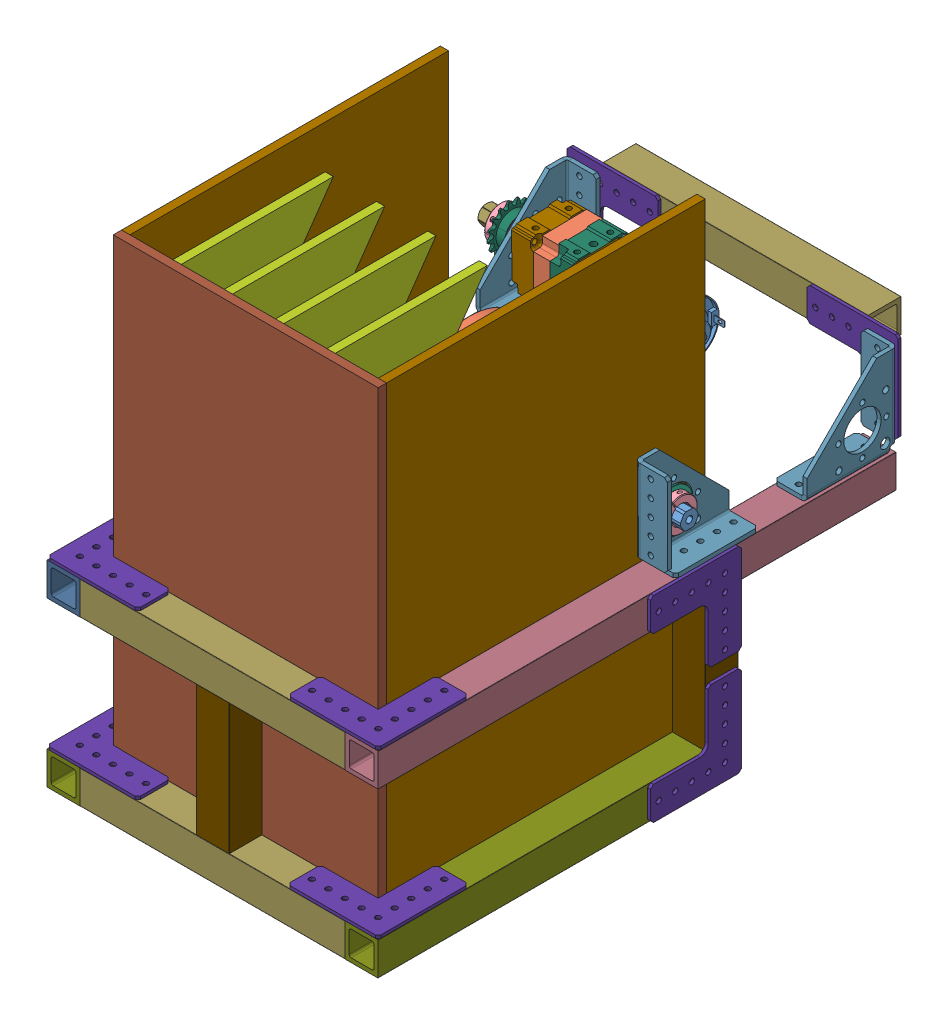
SolidWorks assembly Outtake, configuration Default. Lengths in mm.
Overall size (762 627.63 736.73).
92 component instances, 37 part files, 6 mates.
Components (placement in the parent):
- Skeleton Infinite Recharge Sketch-1: Skeleton Infinite Recharge Sketch [Default] at origin size (762 246.63 736.6)
- Assem_Launch_Component(wheels,hexshaft,motor,etc.)-SP - Copy-1: Assem_Launch_Component(wheels,hexshaft,motor,etc.)-SP - Copy [Default] at (101.6 246.634 342.9) size (290.76 381 426.56)
  - ThunderHex(.5 11inch)-SP-1: ThunderHex(.5 11inch)-SP [Default] at (-34.4752 190.5 -222.25) x (0 0.015634 -0.999878) z (-1 0 0) size (13.74 12.75 279.4)
  - CompliantWheel(4inch 500)SP-1: CompliantWheel(4inch 500)SP [Default] at (-57.548 185.9668 -238.3103) x (0 -0.486399 -0.873737) z (-1 0 0) size (101.6 101.6 25.4)
    - CompliantWheel(4inch 500)SP.STEP-1: CompliantWheel(4inch 500)SP.STEP [Default] at origin size (101.6 101.6 25.4)
      - 4IN Compliant Wheel FINAL Overmold.STEP-1: 4IN Compliant Wheel FINAL Overmold.STEP [Default] at (-16.2374 3.8509 18.652) size (101.6 101.6 25.4)
      - 2in Wheel Intergrated 0500 HEX Hub.STEP-1: 2in Wheel Intergrated 0500 HEX Hub.STEP [Default] at (-16.2374 3.8509 5.952) x (-1 0 0) z (0 0 -1) size (41.91 41.91 25.4)
  - CompliantWheel(4inch 500)SP.STEP-1: CompliantWheel(4inch 500)SP.STEP [Default] at (-82.948 195.0332 -206.1897) x (0 0.486399 0.873737) z (-1 0 0) size (101.6 101.6 25.4)
    - 4IN Compliant Wheel FINAL Overmold.STEP-1: 4IN Compliant Wheel FINAL Overmold.STEP [Default] at (-16.2374 3.8509 18.652) size (101.6 101.6 25.4)
    - 2in Wheel Intergrated 0500 HEX Hub.STEP-1: 2in Wheel Intergrated 0500 HEX Hub.STEP [Default] at (-16.2374 3.8509 5.952) x (-1 0 0) z (0 0 -1) size (41.91 41.91 25.4)
  - CompliantWheel(4inch 500)SP.STEP-3: CompliantWheel(4inch 500)SP.STEP [Default] at (-108.348 195.2838 -206.2625) x (0 0.5 0.866025) z (-1 0 0) size (101.6 101.6 25.4)
    - 4IN Compliant Wheel FINAL Overmold.STEP-1: 4IN Compliant Wheel FINAL Overmold.STEP [Default] at (-16.2374 3.8509 18.652) size (101.6 101.6 25.4)
    - 2in Wheel Intergrated 0500 HEX Hub.STEP-1: 2in Wheel Intergrated 0500 HEX Hub.STEP [Default] at (-16.2374 3.8509 5.952) x (-1 0 0) z (0 0 -1) size (41.91 41.91 25.4)
  - CompliantWheel(4inch 500)SP.STEP-4: CompliantWheel(4inch 500)SP.STEP [Default] at (-133.748 195.0332 -206.1897) x (0 0.486399 0.873737) z (-1 0 0) size (101.6 101.6 25.4)
    - 4IN Compliant Wheel FINAL Overmold.STEP-1: 4IN Compliant Wheel FINAL Overmold.STEP [Default] at (-16.2374 3.8509 18.652) size (101.6 101.6 25.4)
    - 2in Wheel Intergrated 0500 HEX Hub.STEP-1: 2in Wheel Intergrated 0500 HEX Hub.STEP [Default] at (-16.2374 3.8509 5.952) x (-1 0 0) z (0 0 -1) size (41.91 41.91 25.4)
  - ClampingShaftCollar(.5 in)SP-1: ClampingShaftCollar(.5 in)SP [Default] at (-47.625 190.7032 -222.2468) x (0 0.015634 -0.999878) z (-1 0 0) size (25.39 25.4 6.35)
  - ClampingShaftCollar(.5 in)SP-2: ClampingShaftCollar(.5 in)SP [Default] at (-155.575 190.4012 -222.4275) x (0 0.873737 -0.486399) z (-1 0 0) size (25.39 25.4 6.35)
  - VersaPlanetaryv2_Single_Stage_10_1_with_775_Series (General_GearBox_Shell)-SP-1: VersaPlanetaryv2_Single_Stage_10_1_with_775_Series (General_GearBox_Shell)-SP [Default] at (-205.875 214.6824 -345.637) x (-1 0 0) z (0 -0.015634 0.999878) size (166.6 51.28 52.65)
    - VersaPlanetary_v2_Single_Stage_10_1_with_775_Series (General_GearBox_Shell)-SP.STEP-1: VersaPlanetary_v2_Single_Stage_10_1_with_775_Series (General_GearBox_Shell)-SP.STEP [Default] at origin size (166.6 51.28 52.65)
      - 217-2820 Rev1_Public.STEP-1: 217-2820 Rev1_Public.STEP [Default] at (-4.6546 22.225 0) x (0 -0.456494 0.889726) z (-1 0 0) size (39.22 38.88 17.4)
        - 217-2625-100.STEP-1: 217-2625-100.STEP [Default] at origin size (39.22 38.88 12.7)
          - 217-2625-008 Rev1.STEP-1: 217-2625-008 Rev1.STEP [Default] at origin size (34.7 34.7 4.7)
          - 217-2625-010 Rev1.STEP-1: 217-2625-010 Rev1.STEP [Default] at (0 10.193 3.65) x (0.999813 0.019336 0) z (0 0 1) size (4 4 12)
          - 217-2625-010 Rev1.STEP-2: 217-2625-010 Rev1.STEP [Default] at (8.691 -5.3258 3.65) size (4 4 12)
          - 217-2625-010 Rev1.STEP-3: 217-2625-010 Rev1.STEP [Default] at (-8.691 -5.3258 3.65) size (4 4 12)
          - 217-2625-005 Rev1_Planet_Revolving_Follower01.STEP-1: 217-2625-005 Rev1_Planet_Revolving_Follower01.STEP [Default] at (8.691 -5.3258 6.35) x (0.932816 0.360354 0) z (0 0 1) size (16.89 16.89 8)
          - 217-2625-005 Rev1_Planet_Revolving_Follower01.STEP-2: 217-2625-005 Rev1_Planet_Revolving_Follower01.STEP [Default] at (-8.691 -5.3258 6.35) x (-0.932788 -0.360426 0) z (0 0 1) size (16.89 16.89 8)
          - 217-2625-005 Rev1_Planet_Revolving_Follower01.STEP-3: 217-2625-005 Rev1_Planet_Revolving_Follower01.STEP [Default] at (0 10.193 6.35) x (0.893583 0.448898 0) z (0 0 1) size (16.89 16.89 8)
        - 217-2625-007 Rev1_Public.STEP-1: 217-2625-007 Rev1_Public.STEP [Default] at (0 0 6.7) x (0.992772 0.120019 0) z (0 0 1) size (15.27 15.27 12.7)
      - 217-2625-026 Rev1.STEP-1: 217-2625-026 Rev1.STEP [Default] at (-6.5 22.225 0) x (0 -1 0) z (-1 0 0) size (44.45 42 18.12)
      - 217-2742-001 Rev4.STEP-1: 217-2742-001 Rev4.STEP [Default] at (0.2002 22.225 0) x (1 0 0) z (0 -0.092627 0.995701) size (7 28 28)
      - 217-2742-001 Rev4.STEP-2: 217-2742-001 Rev4.STEP [Default] at (8.2002 22.225 0) size (7 28 28)
      - 217-2625-017 Rev1_9714K61.STEP-1: 217-2625-017 Rev1_9714K61.STEP [Default] at (7.42 22.3002 -0.342) x (0 0.56703 0.823697) z (0 -0.823697 0.56703) size (28.51 4.98 27.43)
      - 217-2625-003 Rev1.STEP-1: 217-2625-003 Rev1.STEP [Default] at (7.4478 22.225 0) x (0 -1 0) z (1 0 0) size (17 17 64.11)
      - 217-2625-018 Rev1_98541A410.STEP-1: 217-2625-018 Rev1_98541A410.STEP [Default] at (-0.7046 22.225 0) x (1 0 0) z (0 -0.017452 0.999848) size (1 19.6 17.4)
      - 832-1750-Ring-Gear-Screw_SSA0832-0500ZC.STEP-1: 832-1750-Ring-Gear-Screw_SSA0832-0500ZC.STEP [Default] at (-30.7 4.725 -17.5) x (0 0.997447 0.071411) z (0 -0.071411 0.997447) size (6.73 48.51 6.73)
      - 832-1750-Ring-Gear-Screw_SSA0832-0500ZC.STEP-2: 832-1750-Ring-Gear-Screw_SSA0832-0500ZC.STEP [Default] at (-30.7 39.725 17.5) x (0 0.005929 0.999982) z (0 -0.999982 0.005929) size (6.73 48.51 6.73)
      - 217-2625-025 Rev1.STEP-1: 217-2625-025 Rev1.STEP [Default] at (-23.2 22.225 0) x (0 -1 0) z (-1 0 0) size (44.45 42 18)
      - 217-4649-002 Rev1_SSA0832-0500ZC.STEP-1: 217-4649-002 Rev1_SSA0832-0500ZC.STEP [Default] at (-34.2 4.2645 17.9605) x (0 0.33842 -0.940995) z (0 0.940995 0.33842) size (6.73 16.76 6.73)
      - 217-4649-002 Rev1_SSA0832-0500ZC.STEP-2: 217-4649-002 Rev1_SSA0832-0500ZC.STEP [Default] at (-34.2 40.1855 -17.9605) x (0 -0.308932 -0.951084) z (0 0.951084 -0.308932) size (6.73 16.76 6.73)
      - 217-4649-006 Rev1_SSA0004-008BA.STEP-1: 217-4649-006 Rev1_SSA0004-008BA.STEP [Default] at (-30.7 22.225 14.5) x (0 0.5 -0.866025) z (0 -0.866025 -0.5) size (7 14 7)
      - 217-4649-006 Rev1_SSA0004-008BA.STEP-2: 217-4649-006 Rev1_SSA0004-008BA.STEP [Default] at (-30.7 22.225 -14.5) x (0 -1 0) z (0 0 1) size (7 14 7)
      - 217-2822-002 Rev4.STEP-1: 217-2822-002 Rev4.STEP [Default] at (-32.45 22.225 0) x (0 -1 0) z (-1 0 0) size (42 42 5.3)
      - 217-4347-000 Rev1.STEP-1: 217-4347-000 Rev1.STEP [Default] at (-34.2 22.225 0) x (-1 0 0) z (0 1 0) size (88 44.3 44.3)
      - 217-2816-001 Rev1.STEP-1: 217-2816-001 Rev1.STEP [Default] at (-6.35 22.225 0) x (0 -1 0) z (1 0 0) size (42 42 14.51)
      - 217-4649-001 Rev1.STEP-1: 217-4649-001 Rev1.STEP [Default] at (-20.554 22.225 0) x (0 -1 0) z (1 0 0) size (18 18 13)
      - 217-4649-007 Rev1_94105A824.STEP-1: 217-4649-007 Rev1_94105A824.STEP [Default] at (-26.029 22.225 -6.7835) x (-0.996104 -0.088191 0) z (0 0 -1) size (4.83 4.83 4.77)
      - 217-2625-013 Rev2.STEP-1: 217-2625-013 Rev2.STEP [Default] at (-25.2898 22.225 0) x (0 0 1) z (-1 0 0) size (8.01 7.94 7.5)
  - 13_75mm_1_2_ThunderHex_ID_x_1_125_OD_x_0_313_WD_Flanged_Bearing_217-4006.step-1: 13_75mm_1_2_ThunderHex_ID_x_1_125_OD_x_0_313_WD_Flanged_Bearing_217-4006.step [Default] at (-0.3489 190.5 -222.25) x (0 -0.574166 -0.818739) z (1 0 0) size (31.12 31.12 7.94)
  - betterRamp RC-1: betterRamp RC [Default] at (-39.37 168.0882 -127) x (-1 0 0) z (0 0 -1) size (6.35 381 215.9)
  - betterRamp RC-2: betterRamp RC [Default] at (-118.11 168.0882 -127) x (-1 0 0) z (0 0 -1) size (6.35 381 215.9)
  - betterRamp RC-3: betterRamp RC [Default] at (-78.74 168.0882 -127) x (-1 0 0) z (0 0 -1) size (6.35 381 215.9)
  - betterRamp RC-4: betterRamp RC [Default] at (-157.48 168.0882 -127) x (-1 0 0) z (0 0 -1) size (6.35 381 215.9)
  - ClampingShaftCollar(.5 in)SP-3: ClampingShaftCollar(.5 in)SP [Default] at (6.9517 190.5 -222.25) x (0 0.858103 0.513478) z (-1 0 0) size (25.39 25.4 6.35)
  - ThunderHexFlangedBearing(0.5in) RC-1: ThunderHexFlangedBearing(0.5in) RC [Default] at (-203.9473 190.5 -222.25) x (0 0.030565 0.999533) z (-1 0 0) size (31.12 31.12 7.94)
  - ClampingShaftCollar(.5 in)SP-4: ClampingShaftCollar(.5 in)SP [Default] at (-209.7506 190.5 -222.25) x (0 -0.581767 0.813355) z (-1 0 0) size (25.39 25.4 6.35)
  - Wall(15 by 15 in .125thickness)-SP-2: Wall(15 by 15 in .125thickness)-SP [Default] at (0 190.5 -128.5875) x (-1 0 0) z (0 0 -1) size (6.35 381 244.47)
  - Wall(15 by 15 in .125thickness)-SP-3: Wall(15 by 15 in .125thickness)-SP [Default] at (-203.2 190.5 -128.5875) x (1 0 0) z (0 0 -1) size (6.35 381 244.47)
  - 1x1AluminumStock(15in)-1: 1x1AluminumStock(15in) [Default] at (-228.6 139.7 -1803.4) size (25.4 25.4 419.1)
  - BackWall-SP-1: BackWall-SP [Default] at (311.6896 672.1897 -6.35) size (203.2 381 6.35)
  - 1x1AluminumStock(9.5in)-1: 1x1AluminumStock(9.5in) [Default] at (1625.6 139.7 0) x (0 0 1) z (-1 0 0) size (25.4 25.4 203.2)
  - 1x1AluminumStock(9.5in)-2: 1x1AluminumStock(9.5in) [Default] at (1625.6 215.773 -401.0306) x (0 0 1) z (-1 0 0) size (25.4 25.4 203.2)
  - 1x1AluminumStock(11in)-2: 1x1AluminumStock(11in) [Default] at (25.4 139.7 1457.1726) x (-1 0 0) z (0 0 -1) size (25.4 25.4 397.03)
  - CornerGussetBearingAssem-2: CornerGussetBearingAssem [Default] at (-276.5029 188.5569 -375.7969) x (0 1 0) z (1 0 0) size (69.72 69.72 26.99)
    - CornerGusset-1: CornerGusset [Default] at (-23.4569 2.4523 47.9029) size (69.72 69.72 25.4)
    - ThunderHexFlangedBearing(0.5in) RC-1: ThunderHexFlangedBearing(0.5in) RC [Default] at (3.9032 29.8124 50.2842) x (0.923728 0.383049 0) z (0 0 -1) size (31.12 31.12 7.94)
  - 16AluminumSprocket(#25,0.5inHexBore)-1: 16AluminumSprocket(#25,0.5inHexBore) [Default] at (-242.9193 192.4727 -345.9769) x (0 0.486399 0.873737) z (-1 0 0) size (35.22 35.22 9.18)
  - 16AluminumSprocket(#25,0.5inHexBore)-2: 16AluminumSprocket(#25,0.5inHexBore) [Default] at (-242.9193 190.5254 -222.2496) x (0 -0.486399 -0.873737) z (-1 0 0) size (35.22 35.22 9.18)
  - ClampingShaftCollar(.5 in)SP-5: ClampingShaftCollar(.5 in)SP [Default] at (-233.3625 192.3343 -346.0598) x (0 -0.015634 0.999878) z (-1 0 0) size (25.39 25.4 6.35)
  - 1x1AluminumStock(10.88in)-1: 1x1AluminumStock(10.88in) [Default] at (-228.6 14.2875 -1803.273) size (25.4 25.4 276.35)
  - 1x1AluminumStock(10.88in)-2: 1x1AluminumStock(10.88in) [Default] at (0 14.2875 -1803.273) size (25.4 25.4 276.35)
  - 1x1AluminumStock(9.5in)-3: 1x1AluminumStock(9.5in) [Default] at (1625.6 14.2875 0.127) x (0 0 1) z (-1 0 0) size (25.4 25.4 203.2)
  - ClampingShaftCollar(.5 in)SP-6: ClampingShaftCollar(.5 in)SP [Default] at (-233.3625 190.3975 -222.1929) x (0 0.015634 -0.999878) z (1 0 0) size (25.39 25.4 6.35)
  - ClampingShaftCollar(.5 in)SP-7: ClampingShaftCollar(.5 in)SP [Default] at (-248.8882 190.3993 -222.3102) x (0 -0.015634 0.999878) z (-1 0 0) size (25.39 25.4 6.35)
  - ClampingShaftCollar(.5 in)SP-8: ClampingShaftCollar(.5 in)SP [Default] at (-248.8882 192.332 -345.9131) x (0 -0.015634 0.999878) z (-1 0 0) size (25.39 25.4 6.35)
  - L-Bracket(90degree)-2: L-Bracket(90degree) [Default] at (-216.027 167.386 12.827) x (1 0 0) z (0 -1 0) size (69.6 69.6 2.29)
  - L-Bracket(90degree)-4: L-Bracket(90degree) [Default] at (12.827 39.6875 12.954) x (-1 0 0) z (0 1 0) size (69.6 69.6 2.29)
  - L-Bracket(90degree)-5: L-Bracket(90degree) [Default] at (12.827 165.1 12.827) x (-1 0 0) z (0 1 0) size (69.6 69.6 2.29)
  - L-Bracket(90degree)-6: L-Bracket(90degree) [Default] at (-216.027 41.9735 12.954) x (1 0 0) z (0 -1 0) size (69.6 69.6 2.29)
  - 1x1AluminumStock(3.95in)-1: 1x1AluminumStock(3.95in) [Default] at (-228.6 1868.4875 -250.825) x (1 0 0) z (0 -1 0) size (25.4 25.4 100.08)
  - 1x1AluminumStock(3.95in)-2: 1x1AluminumStock(3.95in) [Default] at (0 1868.4875 -250.825) x (1 0 0) z (0 -1 0) size (25.4 25.4 100.08)
  - 1x1AluminumStock(3.95in)-3: 1x1AluminumStock(3.95in) [Default] at (-114.3 1868.4875 0) x (1 0 0) z (0 -1 0) size (25.4 25.4 100.08)
  - L-Bracket(90degree)-7: L-Bracket(90degree) [Default] at (25.4 26.8605 -238.252) x (0 0 1) z (1 0 0) size (69.6 69.6 2.29)
  - L-Bracket(90degree)-8: L-Bracket(90degree) [Default] at (-230.886 26.8605 -238.252) x (0 0 1) z (1 0 0) size (69.6 69.6 2.29)
  - L-Bracket(90degree)-9: L-Bracket(90degree) [Default] at (25.4 152.527 -238.252) x (0 -1 0) z (1 0 0) size (69.6 69.6 2.29)
  - L-Bracket(90degree)-10: L-Bracket(90degree) [Default] at (-230.886 152.527 -238.252) x (0 -1 0) z (1 0 0) size (69.6 69.6 2.29)
  - CornerGusset-1: CornerGusset [Default] at (0 165.1 -196.2958) x (0 0 -1) z (1 0 0) size (69.72 69.72 25.4)
  - CornerGusset-2: CornerGusset [Default] at (-203.2 165.1 -195.1148) x (0 1 0) z (-1 0 0) size (69.72 69.72 25.4)
  - CornerGusset-3: CornerGusset [Default] at (25.4 165.1 -373.3446) x (0 0 1) z (-1 0 0) size (69.72 69.72 25.4)
  - L-Bracket(90degree)-11: L-Bracket(90degree) [Default] at (12.7 228.6 -375.6306) x (0 -1 0) z (0 0 1) size (69.6 69.6 2.29)
  - L-Bracket(90degree)-12: L-Bracket(90degree) [Default] at (-215.9 228.6 -375.6306) size (69.6 69.6 2.29)
Mates (geometry in assembly coordinates):
- Coincident1: coincident aligned: plane of Skeleton Infinite Recharge Sketch-1 through (0 246.634 0) normal (0 1 0); plane of Assem_Launch_Component(wheels,hexshaft,motor,etc.)-SP - Copy-1 through (101.6 246.634 342.9) normal (0 1 0)
- Coincident2: coincident aligned: plane of Skeleton Infinite Recharge Sketch-1 through (0 0 0) normal (0 0 1); plane of assembly through (0 0 0) normal (0 0 1)
- Coincident3: coincident aligned: plane of Skeleton Infinite Recharge Sketch-1 through (0 0 0) normal (0 1 0); plane of assembly through (0 0 0) normal (0 1 0)
- Coincident4: coincident aligned: plane of Skeleton Infinite Recharge Sketch-1 through (0 0 0) normal (1 0 0); plane of assembly through (0 0 0) normal (1 0 0)
- Coincident5: coincident anti-aligned: line of Skeleton Infinite Recharge Sketch-1 through (0 246.634 -368.3) axis (0 0 1); line of Assem_Launch_Component(wheels,hexshaft,motor,etc.)-SP - Copy-1 through (0 246.634 368.3) axis (0 0 -1)
- Coincident6: coincident aligned: line of Skeleton Infinite Recharge Sketch-1 through (-95.25 246.634 368.3) axis (1 0 0); line of Assem_Launch_Component(wheels,hexshaft,motor,etc.)-SP - Copy-1 through (-127 246.634 368.3) axis (1 0 0)
